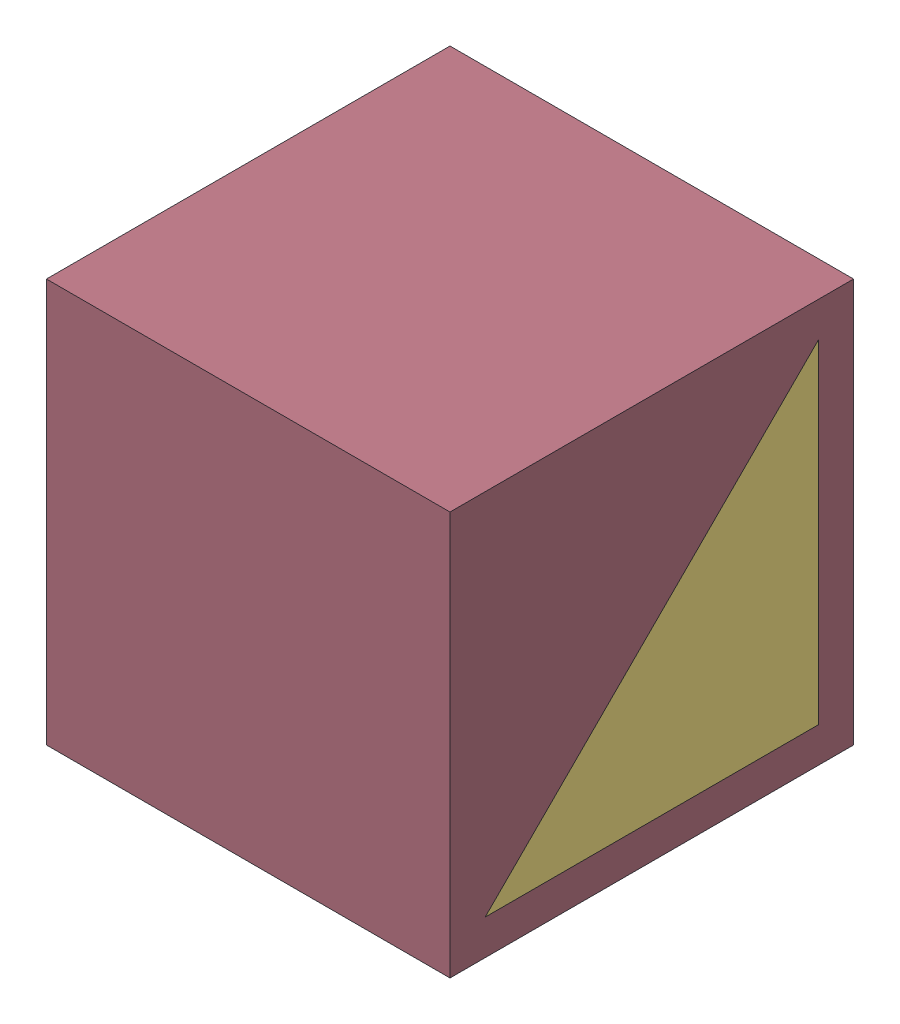
SolidWorks assembly cube_, configuration cube05. Lengths in mm.
Overall size (127.64 127.64 127.64).
31 component instances, 31 part files, 93 mates.
Components (placement in the parent):
- pr^cube_-28: pr^cube_ [cube01] x (-1 0 0) z (0 0 1) size (105.41 1.59 105.41) (virtual)
- pg^cube_-20: pg^cube_ [cube01] x (0 -1 0) z (0 0 1) size (105.41 1.59 105.41) (virtual)
- po^cube_-22: po^cube_ [cube01] x (0 1 0) z (0 0 1) size (105.41 1.59 105.41) (virtual)
- py^cube_-21: py^cube_ [cube01] at origin size (105.41 1.59 105.41) (virtual)
- pc^cube_-18: pc^cube_ [cube01] x (-1 0 0) z (0 -1 0) size (105.41 1.59 105.41) (virtual)
- pb^cube_-21: pb^cube_ [cube01] x (-1 0 0) z (0 1 0) size (105.41 1.59 105.41) (virtual)
- br1^cube_-49: br1^cube_ [Default] at (0 36.83 -36.83) x (0 0 1) z (-1 0 0) size (50.8 50.8 66.55) (virtual)
- br2^cube_-61: br2^cube_ [Default] at (-36.83 36.83 0) size (50.8 50.8 66.55) (virtual)
- br3^cube_-46: br3^cube_ [Default] at (0 36.83 36.83) x (0 0 -1) z (1 0 0) size (50.8 50.8 66.55) (virtual)
- bg1^cube_-47: bg1^cube_ [Default] at (-36.83 -36.83 0) x (0 1 0) z (0 0 1) size (50.8 50.8 66.55) (virtual)
- bg2^cube_-44: bg2^cube_ [Default] at (-36.83 0 36.83) x (0 0 -1) z (0 1 0) size (50.8 50.8 66.55) (virtual)
- bg3^cube_-40: bg3^cube_ [Default] at (-36.83 0 -36.83) x (0 0 1) z (0 -1 0) size (50.8 50.8 66.55) (virtual)
- bo1^cube_-42: bo1^cube_ [Default] at (36.83 0 -36.83) x (0 0 1) z (0 1 0) size (50.8 50.8 66.55) (virtual)
- bo2^cube_-46: bo2^cube_ [Default] at (36.83 0 36.83) x (0 0 -1) z (0 -1 0) size (50.8 50.8 66.55) (virtual)
- bo3^cube_-62: bo3^cube_ [Default] at (36.83 36.83 0) x (0 -1 0) z (0 0 1) size (50.8 50.8 66.55) (virtual)
- by1^cube_-41: by1^cube_ [Default] at (0 -36.83 -36.83) x (0 0 1) z (1 0 0) size (50.8 50.8 66.55) (virtual)
- by2^cube_-45: by2^cube_ [Default] at (0 -36.83 36.83) x (0 0 -1) z (-1 0 0) size (50.8 50.8 66.55) (virtual)
- by3^cube_-48: by3^cube_ [Default] at (36.83 -36.83 0) x (-1 0 0) z (0 0 1) size (50.8 50.8 66.55) (virtual)
- dr1^cube_-55: dr1^cube_ [cube01] at (-61.6246 62.23 0) x (0 -1 0) z (0 0 1) size (26.01 26.01 124.47) (virtual)
- dr2^cube_-37: dr2^cube_ [cube01] at (0 62.23 61.6246) x (0 -1 0) z (1 0 0) size (26.01 26.01 124.47) (virtual)
- dr3^cube_-33: dr3^cube_ [cube01] at (0 62.23 -61.6246) x (0 -1 0) z (-1 0 0) size (26.01 26.01 124.47) (virtual)
- dg1^cube_-38: dg1^cube_ [cube01] at (-62.23 0 61.6246) x (1 0 0) z (0 1 0) size (26.01 26.01 124.47) (virtual)
- dg2^cube_-41: dg2^cube_ [cube01] at (-62.23 -61.6246 0) size (26.01 26.01 124.47) (virtual)
- dg3^cube_-34: dg3^cube_ [cube01] at (-62.23 0 -61.6246) x (1 0 0) z (0 -1 0) size (26.01 26.01 124.47) (virtual)
- do3^cube_-47: do3^cube_ [cube01] at (62.23 61.6246 0) x (-1 0 0) z (0 0 1) size (26.01 26.01 124.47) (virtual)
- do1^cube_-36: do1^cube_ [cube01] at (62.23 0 -61.6246) x (-1 0 0) z (0 1 0) size (26.01 26.01 124.47) (virtual)
- do2^cube_-40: do2^cube_ [cube01] at (62.23 0 61.6246) x (-1 0 0) z (0 -1 0) size (26.01 26.01 124.47) (virtual)
- dy1^cube_-35: dy1^cube_ [cube01] at (0 -62.23 -61.6246) x (0 1 0) z (1 0 0) size (26.01 26.01 124.47) (virtual)
- dy2^cube_-39: dy2^cube_ [cube01] at (0 -62.23 61.6246) x (0 1 0) z (-1 0 0) size (26.01 26.01 124.47) (virtual)
- dy3^cube_-42: dy3^cube_ [cube01] at (61.6246 -62.23 0) x (0 1 0) z (0 0 1) size (26.01 26.01 124.47) (virtual)
- boundry^cube_-1: boundry^cube_ [Default] at origin size (127.64 127.64 127.64) (virtual)
Mates (geometry in assembly coordinates):
- Coincident1: coincident anti-aligned: plane of pr^cube_-28 through (52.705 62.23 -52.705) normal (0 -1 0); plane of br1^cube_-49 through (-33.274 62.23 -36.83) normal (0 1 0)
- Coincident2: coincident anti-aligned: plane of pr^cube_-28 through (52.705 62.23 -52.705) normal (0 -1 0); plane of br2^cube_-61 through (-36.83 62.23 33.274) normal (0 1 0)
- Coincident3: coincident anti-aligned: plane of pr^cube_-28 through (52.705 62.23 -52.705) normal (0 -1 0); plane of br3^cube_-46 through (33.274 62.23 36.83) normal (0 1 0)
- Coincident4: coincident anti-aligned: plane of pr^cube_-28 through (52.705 62.23 -52.705) normal (0 -1 0); plane of bo3^cube_-62 through (36.83 62.23 33.274) normal (0 1 0)
- Coincident5: coincident anti-aligned: plane of pr^cube_-28 through (52.705 62.23 -52.705) normal (0 -1 0); plane of dr3^cube_-33 through (0 62.23 -123.8546) normal (0 1 0)
- Coincident6: coincident anti-aligned: plane of pr^cube_-28 through (52.705 62.23 -52.705) normal (0 -1 0); plane of dr1^cube_-55 through (-123.8546 62.23 0) normal (0 1 0)
- Coincident7: coincident anti-aligned: plane of pr^cube_-28 through (52.705 62.23 -52.705) normal (0 -1 0); plane of do3^cube_-47 through (-0.6054 62.23 0) normal (0 1 0)
- Coincident8: coincident anti-aligned: plane of pr^cube_-28 through (52.705 62.23 -52.705) normal (0 -1 0); plane of dr2^cube_-37 through (0 62.23 123.8546) normal (0 1 0)
- Coincident34: coincident anti-aligned: plane of pb^cube_-21 through (52.705 -52.705 -62.23) normal (0 0 1); plane of by1^cube_-41 through (33.274 -36.83 -62.23) normal (0 0 -1)
- Coincident35: coincident anti-aligned: plane of pb^cube_-21 through (52.705 -52.705 -62.23) normal (0 0 1); plane of bo1^cube_-42 through (36.83 33.274 -62.23) normal (0 0 -1)
- Coincident36: coincident anti-aligned: plane of pb^cube_-21 through (52.705 -52.705 -62.23) normal (0 0 1); plane of br1^cube_-49 through (-33.274 36.83 -62.23) normal (0 0 -1)
- Coincident37: coincident anti-aligned: plane of pb^cube_-21 through (52.705 -52.705 -62.23) normal (0 0 1); plane of bg3^cube_-40 through (-36.83 -33.274 -62.23) normal (0 0 -1)
- Coincident38: coincident anti-aligned: plane of pb^cube_-21 through (52.705 -52.705 -62.23) normal (0 0 1); plane of dg3^cube_-34 through (0.6054 0 -62.23) normal (0 0 -1)
- Coincident39: coincident anti-aligned: plane of pb^cube_-21 through (52.705 -52.705 -62.23) normal (0 0 1); plane of dr3^cube_-33 through (0 -0.6054 -62.23) normal (0 0 -1)
- Coincident40: coincident anti-aligned: plane of pb^cube_-21 through (52.705 -52.705 -62.23) normal (0 0 1); plane of do1^cube_-36 through (-0.6054 0 -62.23) normal (0 0 -1)
- Coincident41: coincident anti-aligned: plane of pb^cube_-21 through (52.705 -52.705 -62.23) normal (0 0 1); plane of dy1^cube_-35 through (0 0.6054 -62.23) normal (0 0 -1)
- Coincident42: coincident anti-aligned: plane of pc^cube_-18 through (52.705 52.705 62.23) normal (0 0 -1); plane of bo2^cube_-46 through (36.83 -33.274 62.23) normal (0 0 1)
- Coincident43: coincident anti-aligned: plane of pc^cube_-18 through (52.705 52.705 62.23) normal (0 0 -1); plane of br3^cube_-46 through (33.274 36.83 62.23) normal (0 0 1)
- Coincident44: coincident anti-aligned: plane of pc^cube_-18 through (52.705 52.705 62.23) normal (0 0 -1); plane of bg2^cube_-44 through (-36.83 33.274 62.23) normal (0 0 1)
- Coincident45: coincident anti-aligned: plane of pc^cube_-18 through (52.705 52.705 62.23) normal (0 0 -1); plane of by2^cube_-45 through (-33.274 -36.83 62.23) normal (0 0 1)
- Coincident46: coincident anti-aligned: plane of pc^cube_-18 through (52.705 52.705 62.23) normal (0 0 -1); plane of do2^cube_-40 through (-0.6054 0 62.23) normal (0 0 1)
- Coincident47: coincident anti-aligned: plane of pc^cube_-18 through (52.705 52.705 62.23) normal (0 0 -1); plane of dy2^cube_-39 through (0 0.6054 62.23) normal (0 0 1)
- Coincident48: coincident anti-aligned: plane of pc^cube_-18 through (52.705 52.705 62.23) normal (0 0 -1); plane of dg1^cube_-38 through (0.6054 0 62.23) normal (0 0 1)
- Coincident49: coincident anti-aligned: plane of pc^cube_-18 through (52.705 52.705 62.23) normal (0 0 -1); plane of dr2^cube_-37 through (0 -0.6054 62.23) normal (0 0 1)
- Coincident50: coincident anti-aligned: plane of pg^cube_-20 through (-62.23 52.705 -52.705) normal (1 0 0); plane of bg3^cube_-40 through (-62.23 -33.274 -36.83) normal (-1 0 0)
- Coincident51: coincident anti-aligned: plane of pg^cube_-20 through (-62.23 52.705 -52.705) normal (1 0 0); plane of bg1^cube_-47 through (-62.23 -36.83 33.274) normal (-1 0 0)
- Coincident52: coincident anti-aligned: plane of pg^cube_-20 through (-62.23 52.705 -52.705) normal (1 0 0); plane of bg2^cube_-44 through (-62.23 33.274 36.83) normal (-1 0 0)
- Coincident53: coincident anti-aligned: plane of pg^cube_-20 through (-62.23 52.705 -52.705) normal (1 0 0); plane of dr1^cube_-55 through (-62.23 -0.6054 0) normal (-1 0 0)
- Coincident54: coincident anti-aligned: plane of pg^cube_-20 through (-62.23 52.705 -52.705) normal (1 0 0); plane of dg3^cube_-34 through (-62.23 0 -123.8546) normal (-1 0 0)
- Coincident55: coincident anti-aligned: plane of pg^cube_-20 through (-62.23 52.705 -52.705) normal (1 0 0); plane of dg2^cube_-41 through (-62.23 -123.8546 0) normal (-1 0 0)
- Coincident56: coincident anti-aligned: plane of pg^cube_-20 through (-62.23 52.705 -52.705) normal (1 0 0); plane of dg1^cube_-38 through (-62.23 0 123.8546) normal (-1 0 0)
- Coincident99: coincident anti-aligned: plane of pg^cube_-20 through (-62.23 52.705 -52.705) normal (1 0 0); plane of br2^cube_-61 through (-62.23 36.83 33.274) normal (-1 0 0)
- Coincident57: coincident anti-aligned: plane of py^cube_-21 through (-52.705 -62.23 -52.705) normal (0 1 0); plane of by3^cube_-48 through (36.83 -62.23 33.274) normal (0 -1 0)
- Coincident58: coincident anti-aligned: plane of py^cube_-21 through (-52.705 -62.23 -52.705) normal (0 1 0); plane of by2^cube_-45 through (-33.274 -62.23 36.83) normal (0 -1 0)
- Coincident59: coincident anti-aligned: plane of py^cube_-21 through (-52.705 -62.23 -52.705) normal (0 1 0); plane of bg1^cube_-47 through (-36.83 -62.23 33.274) normal (0 -1 0)
- Coincident60: coincident anti-aligned: plane of py^cube_-21 through (-52.705 -62.23 -52.705) normal (0 1 0); plane of by1^cube_-41 through (33.274 -62.23 -36.83) normal (0 -1 0)
- Coincident61: coincident anti-aligned: plane of py^cube_-21 through (-52.705 -62.23 -52.705) normal (0 1 0); plane of dy3^cube_-42 through (123.8546 -62.23 0) normal (0 -1 0)
- Coincident62: coincident anti-aligned: plane of py^cube_-21 through (-52.705 -62.23 -52.705) normal (0 1 0); plane of dy2^cube_-39 through (0 -62.23 123.8546) normal (0 -1 0)
- Coincident63: coincident anti-aligned: plane of py^cube_-21 through (-52.705 -62.23 -52.705) normal (0 1 0); plane of dg2^cube_-41 through (0.6054 -62.23 0) normal (0 -1 0)
- Coincident64: coincident anti-aligned: plane of py^cube_-21 through (-52.705 -62.23 -52.705) normal (0 1 0); plane of dy1^cube_-35 through (0 -62.23 -123.8546) normal (0 -1 0)
- Coincident65: coincident anti-aligned: plane of po^cube_-22 through (62.23 -52.705 -52.705) normal (-1 0 0); plane of bo1^cube_-42 through (62.23 33.274 -36.83) normal (1 0 0)
- Coincident66: coincident anti-aligned: plane of po^cube_-22 through (62.23 -52.705 -52.705) normal (-1 0 0); plane of by3^cube_-48 through (62.23 -36.83 33.274) normal (1 0 0)
- Coincident67: coincident anti-aligned: plane of po^cube_-22 through (62.23 -52.705 -52.705) normal (-1 0 0); plane of bo2^cube_-46 through (62.23 -33.274 36.83) normal (1 0 0)
- Coincident68: coincident anti-aligned: plane of po^cube_-22 through (62.23 -52.705 -52.705) normal (-1 0 0); plane of bo3^cube_-62 through (62.23 36.83 33.274) normal (1 0 0)
- Coincident69: coincident anti-aligned: plane of po^cube_-22 through (62.23 -52.705 -52.705) normal (-1 0 0); plane of do2^cube_-40 through (62.23 0 123.8546) normal (1 0 0)
- Coincident70: coincident anti-aligned: plane of po^cube_-22 through (62.23 -52.705 -52.705) normal (-1 0 0); plane of do3^cube_-47 through (62.23 123.8546 0) normal (1 0 0)
- Coincident71: coincident anti-aligned: plane of po^cube_-22 through (62.23 -52.705 -52.705) normal (-1 0 0); plane of do1^cube_-36 through (62.23 0 -123.8546) normal (1 0 0)
- Coincident72: coincident anti-aligned: plane of po^cube_-22 through (62.23 -52.705 -52.705) normal (-1 0 0); plane of dy3^cube_-42 through (62.23 0.6054 0) normal (1 0 0)
- Coincident73: coincident aligned: plane of assembly through (0 0 0) normal (0 0 1); plane of dy3^cube_-42 through (61.6246 -62.23 0) normal (0 0 1)
- Coincident74: coincident aligned: plane of assembly through (0 0 0) normal (0 0 1); plane of by3^cube_-48 through (36.83 -36.83 0) normal (0 0 1)
- Coincident75: coincident aligned: plane of assembly through (0 0 0) normal (0 0 1); plane of bo3^cube_-62 through (36.83 36.83 0) normal (0 0 1)
- Coincident76: coincident aligned: plane of assembly through (0 0 0) normal (0 0 1); plane of do3^cube_-47 through (62.23 61.6246 0) normal (0 0 1)
- Coincident77: coincident aligned: plane of assembly through (0 0 0) normal (0 0 1); plane of dg2^cube_-41 through (-62.23 -61.6246 0) normal (0 0 1)
- Coincident78: coincident aligned: plane of assembly through (0 0 0) normal (0 0 1); plane of bg1^cube_-47 through (-36.83 -36.83 0) normal (0 0 1)
- Coincident79: coincident aligned: plane of assembly through (0 0 0) normal (0 0 1); plane of dr1^cube_-55 through (-61.6246 62.23 0) normal (0 0 1)
- Coincident80: coincident aligned: plane of assembly through (0 0 0) normal (0 0 1); plane of br2^cube_-61 through (-36.83 36.83 0) normal (0 0 1)
- Coincident81: coincident aligned: plane of assembly through (0 0 0) normal (0 1 0); plane of bo1^cube_-42 through (36.83 0 -36.83) normal (0 1 0)
- Coincident82: coincident aligned: plane of assembly through (0 0 0) normal (0 1 0); plane of py^cube_-21 through (0 0 0) normal (0 1 0)
- Coincident83: coincident aligned: plane of assembly through (0 0 0) normal (0 1 0); plane of do1^cube_-36 through (62.23 0 -61.6246) normal (0 1 0)
- Coincident84: coincident anti-aligned: plane of assembly through (0 0 0) normal (0 1 0); plane of bg3^cube_-40 through (-36.83 0 -36.83) normal (0 -1 0)
- Coincident85: coincident anti-aligned: plane of assembly through (0 0 0) normal (0 1 0); plane of dg3^cube_-34 through (-62.23 0 -61.6246) normal (0 -1 0)
- Coincident86: coincident aligned: plane of assembly through (0 0 0) normal (0 1 0); plane of dg1^cube_-38 through (-62.23 0 61.6246) normal (0 1 0)
- Coincident87: coincident aligned: plane of assembly through (0 0 0) normal (0 1 0); plane of bg2^cube_-44 through (-36.83 0 36.83) normal (0 1 0)
- Coincident88: coincident anti-aligned: plane of assembly through (0 0 0) normal (0 1 0); plane of bo2^cube_-46 through (36.83 0 36.83) normal (0 -1 0)
- Coincident89: coincident anti-aligned: plane of assembly through (0 0 0) normal (0 1 0); plane of do2^cube_-40 through (62.23 0 61.6246) normal (0 -1 0)
- Coincident90: coincident anti-aligned: plane of assembly through (0 0 0) normal (1 0 0); plane of by2^cube_-45 through (0 -36.83 36.83) normal (-1 0 0)
- Coincident91: coincident anti-aligned: plane of assembly through (0 0 0) normal (1 0 0); plane of dy2^cube_-39 through (0 -62.23 61.6246) normal (-1 0 0)
- Coincident92: coincident aligned: plane of assembly through (0 0 0) normal (1 0 0); plane of pg^cube_-20
- Coincident93: coincident aligned: plane of assembly through (0 0 0) normal (1 0 0); plane of dr2^cube_-37 through (0 62.23 61.6246) normal (1 0 0)
- Coincident94: coincident aligned: plane of assembly through (0 0 0) normal (1 0 0); plane of br3^cube_-46 through (0 36.83 36.83) normal (1 0 0)
- Coincident95: coincident anti-aligned: plane of assembly through (0 0 0) normal (1 0 0); plane of dr3^cube_-33 through (0 62.23 -61.6246) normal (-1 0 0)
- Coincident96: coincident anti-aligned: plane of assembly through (0 0 0) normal (1 0 0); plane of br1^cube_-49 through (0 36.83 -36.83) normal (-1 0 0)
- Coincident97: coincident aligned: plane of assembly through (0 0 0) normal (1 0 0); plane of by1^cube_-41 through (0 -36.83 -36.83) normal (1 0 0)
- Coincident98: coincident aligned: plane of assembly through (0 0 0) normal (1 0 0); plane of dy1^cube_-35 through (0 -62.23 -61.6246) normal (1 0 0)
- Coincident100: coincident anti-aligned: plane of pr^cube_-28; plane of assembly through (0 0 0) normal (1 0 0)
- Coincident101: coincident aligned: plane of pr^cube_-28 through (0 0 0) normal (0 0 1); plane of assembly through (0 0 0) normal (0 0 1)
- Coincident102: coincident anti-aligned: plane of pr^cube_-28; plane of assembly through (0 0 0) normal (0 1 0)
- Coincident106: coincident anti-aligned: plane of pg^cube_-20; plane of assembly through (0 0 0) normal (0 1 0)
- Coincident107: coincident aligned: plane of pg^cube_-20; plane of assembly through (0 0 0) normal (1 0 0)
- Coincident108: coincident aligned: plane of pg^cube_-20 through (0 0 0) normal (0 0 1); plane of assembly through (0 0 0) normal (0 0 1)
- Coincident109: coincident aligned: plane of py^cube_-21 through (0 0 0) normal (0 0 1); plane of assembly through (0 0 0) normal (0 0 1)
- Coincident110: coincident aligned: plane of py^cube_-21 through (0 0 0) normal (0 1 0); plane of assembly through (0 0 0) normal (0 1 0)
- Coincident111: coincident aligned: plane of py^cube_-21 through (0 0 0) normal (1 0 0); plane of assembly through (0 0 0) normal (1 0 0)
- Coincident112: coincident aligned: plane of po^cube_-22 through (0 0 0) normal (0 0 1); plane of assembly through (0 0 0) normal (0 0 1)
- Coincident113: coincident anti-aligned: plane of po^cube_-22; plane of assembly through (0 0 0) normal (1 0 0)
- Coincident114: coincident aligned: plane of po^cube_-22; plane of assembly through (0 0 0) normal (0 1 0)
- Coincident115: coincident anti-aligned: plane of pc^cube_-18 through (0 0 0) normal (0 -1 0); plane of assembly through (0 0 0) normal (0 1 0)
- Coincident116: coincident anti-aligned: plane of pc^cube_-18; plane of assembly through (0 0 0) normal (0 0 1)
- Coincident117: coincident anti-aligned: plane of pc^cube_-18; plane of assembly through (0 0 0) normal (1 0 0)
- Coincident118: coincident aligned: plane of pb^cube_-21 through (0 0 0) normal (0 1 0); plane of assembly through (0 0 0) normal (0 1 0)
- Coincident119: coincident aligned: plane of pb^cube_-21; plane of assembly through (0 0 0) normal (0 0 1)
- Coincident120: coincident anti-aligned: line of pb^cube_-21 through (0.8731 -0.8731 0) axis (0 0 -1); sketch_entity of pr^cube_-28; plane of pb^cube_-21 through (52.705 -52.705 -63.8175) normal (0 0 -1); plane of ? through (-52.705 -63.8175 -52.705) normal (0 -1 0)
- cyan_cut: unknown: unknown of pc^cube_-18; plane of pc^cube_-18 through (52.705 52.705 63.8175) normal (0 0 1); plane of pg^cube_-20 through (-63.8175 52.705 -52.705) normal (-1 0 0); plane of po^cube_-22 through (63.8175 -52.705 -52.705) normal (1 0 0); unknown of pr^cube_-28; unknown of ?
